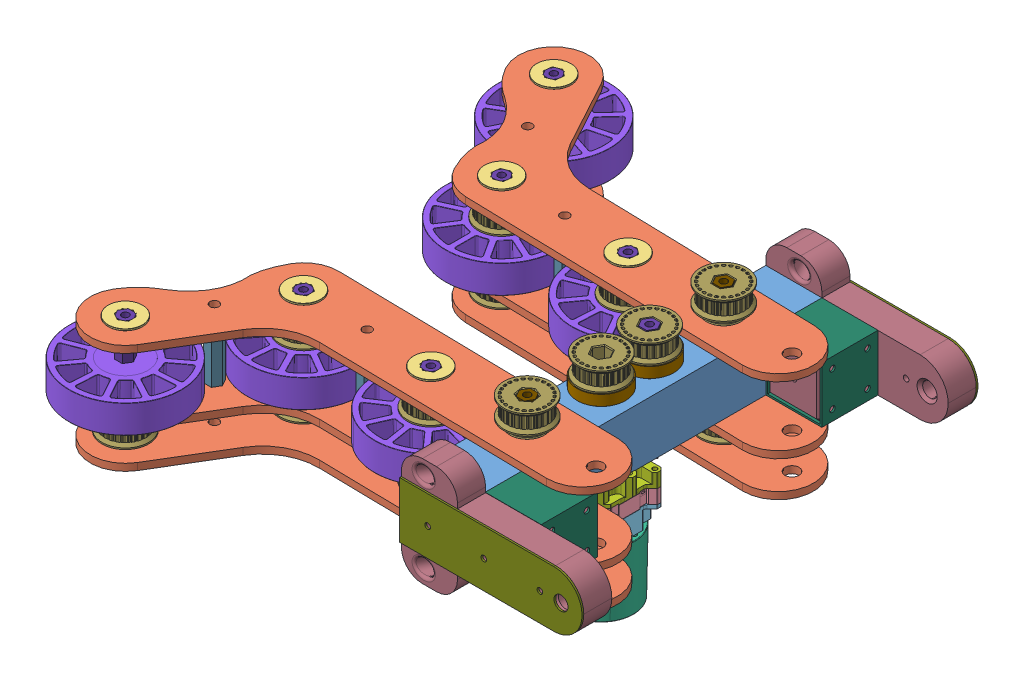
SolidWorks assembly Intake_Claw_1.0, configuration Default. Lengths in mm.
Overall size (476.14 191.6 522.56).
116 component instances, 18 part files, 232 mates.
Components (placement in the parent):
- Claw_Crossbar-1: Claw_Crossbar [Default] at origin size (50.8 50.8 304.8)
- Claw_Intake_Plates-3: Claw_Intake_Plates [Default] at (-63.4848 52.3773 239.6573) x (0.018478 0 -0.999829) z (0.999829 0 0.018478) size (165.24 6.35 379.41)
- am-2986 FR8ZZ Hex Bearing.step-1: am-2986 FR8ZZ Hex Bearing.step [Default] at (25.4 44.3967 241.3) x (-0.023449 0 -0.999725) z (0 1 0) size (31.12 31.12 7.93)
- am-2986 FR8ZZ Hex Bearing.step-3: am-2986 FR8ZZ Hex Bearing.step [Default] at (-241.5471 52.324 338.1202) x (0 0 -1) z (0 1 0) size (31.12 31.12 7.93)
- am-2986 FR8ZZ Hex Bearing.step-5: am-2986 FR8ZZ Hex Bearing.step [Default] at (25.4 52.324 241.3) x (0 0 -1) z (0 1 0) size (31.12 31.12 7.93)
- am-2986 FR8ZZ Hex Bearing.step-11: am-2986 FR8ZZ Hex Bearing.step [Default] at (-63.4848 52.324 239.6573) x (0 0 -1) z (0 1 0) size (31.12 31.12 7.93)
- am-2986 FR8ZZ Hex Bearing.step-12: am-2986 FR8ZZ Hex Bearing.step [Default] at (-180.9398 52.324 237.4866) x (0 0 -1) z (0 1 0) size (31.12 31.12 7.93)
- Intake_Plate_Assembly-1: Intake_Plate_Assembly [Default] at (-25.3851 110.6877 261.8842) x (0.99204 0 0.125922) z (0.125922 0 -0.99204) size (394.05 7.93 202.39)
  - Claw_Intake_Plates-3: Claw_Intake_Plates [Default] at (-63.0534 112.2651 194.2998) x (0.100115 0 -0.994976) z (0.994976 0 0.100115) size (165.24 6.35 379.41)
  - am-2986 FR8ZZ Hex Bearing.step-3: am-2986 FR8ZZ Hex Bearing.step [Default] at (-248.5659 112.2117 277.8835) x (0 0 -1) z (0 1 0) size (31.12 31.12 7.93)
  - am-2986 FR8ZZ Hex Bearing.step-5: am-2986 FR8ZZ Hex Bearing.step [Default] at (25.4 112.2117 203.2) x (0 0 -1) z (0 1 0) size (31.12 31.12 7.93)
  - am-2986 FR8ZZ Hex Bearing.step-11: am-2986 FR8ZZ Hex Bearing.step [Default] at (-63.0534 112.2117 194.2998) x (0 0 -1) z (0 1 0) size (31.12 31.12 7.93)
  - am-2986 FR8ZZ Hex Bearing.step-12: am-2986 FR8ZZ Hex Bearing.step [Default] at (-179.9381 112.2117 182.5388) x (0 0 -1) z (0 1 0) size (31.12 31.12 7.93)
- Intake_Plate_Assembly_2-1: Intake_Plate_Assembly_2 [Default] at (-16.4979 -120.1924 40.8533) x (0.996656 0 -0.081713) z (0.081713 0 0.996656) size (394.05 7.93 202.39)
  - Claw_Intake_Plates-3: Claw_Intake_Plates [Default] at (-63.0746 112.2651 194.2998) x (0.100115 0 -0.994976) z (0.994976 0 0.100115) size (165.24 6.35 379.41)
  - am-2986 FR8ZZ Hex Bearing.step-11: am-2986 FR8ZZ Hex Bearing.step [Default] at (-63.0746 118.6684 194.2998) x (0 0 -1) z (0 -1 0) size (31.12 31.12 7.93)
  - am-2986 FR8ZZ Hex Bearing.step-16: am-2986 FR8ZZ Hex Bearing.step [Default] at (25.3787 118.6684 203.2) x (0 0 -1) z (0 -1 0) size (31.12 31.12 7.93)
  - am-2986 FR8ZZ Hex Bearing.step-17: am-2986 FR8ZZ Hex Bearing.step [Default] at (-179.9594 118.6684 182.5388) x (0 0 -1) z (0 -1 0) size (31.12 31.12 7.93)
  - am-2986 FR8ZZ Hex Bearing.step-18: am-2986 FR8ZZ Hex Bearing.step [Default] at (-248.5872 118.6684 277.8835) x (0 0 -1) z (0 -1 0) size (31.12 31.12 7.93)
- Intake_Plate_Assembly_2-2: Intake_Plate_Assembly_2 [Default] at (-25.364 170.9924 261.8868) x (0.99204 0 0.125922) z (0.125922 0 -0.99204) size (394.05 7.93 202.39)
  - Claw_Intake_Plates-3: Claw_Intake_Plates [Default] at (-63.0746 112.2651 194.2998) x (0.100115 0 -0.994976) z (0.994976 0 0.100115) size (165.24 6.35 379.41)
  - am-2986 FR8ZZ Hex Bearing.step-11: am-2986 FR8ZZ Hex Bearing.step [Default] at (-63.0746 118.6684 194.2998) x (0 0 -1) z (0 -1 0) size (31.12 31.12 7.93)
  - am-2986 FR8ZZ Hex Bearing.step-16: am-2986 FR8ZZ Hex Bearing.step [Default] at (25.3787 118.6684 203.2) x (0 0 -1) z (0 -1 0) size (31.12 31.12 7.93)
  - am-2986 FR8ZZ Hex Bearing.step-17: am-2986 FR8ZZ Hex Bearing.step [Default] at (-179.9594 118.6684 182.5388) x (0 0 -1) z (0 -1 0) size (31.12 31.12 7.93)
  - am-2986 FR8ZZ Hex Bearing.step-18: am-2986 FR8ZZ Hex Bearing.step [Default] at (-248.5872 118.6684 277.8835) x (0 0 -1) z (0 -1 0) size (31.12 31.12 7.93)
- REV-21-2103.step-1: REV-21-2103.step [Default] at (25.4 -25.0519 174.244) x (1 0 0) z (0 1 0) size (61.91 50.8 16.85)
- REV-21-2106.step-1: REV-21-2106.step [Default] at (25.4 -40.9269 174.244) x (1 0 0) z (0 1 0) size (61.91 50.8 19.05)
- REV-21-1650-V1.1.step-1: REV-21-1650-V1.1.step [Default] at (25.4 -50.4519 174.244) x (0.832107 0 0.554615) z (0 1 0) size (68.13 68.01 93.35)
- REV-21-2104.step-1: REV-21-2104.step [Default] at (25.4 -9.1769 174.244) x (0 1 0) z (-1 0 0) size (23.2 50.8 61.92)
- am-3480 4IN 500Hex Bore Compliant Wheel REV2.STEP-1: am-3480 4IN 500Hex Bore Compliant Wheel REV2.STEP [Default] at (-229.2406 20.303 326.8494) x (0.873407 0 -0.486991) z (0 -1 0) size (101.6 101.6 25.4)
- am-3480 4IN 500Hex Bore Compliant Wheel REV2.STEP-2: am-3480 4IN 500Hex Bore Compliant Wheel REV2.STEP [Default] at (-176.0869 20.303 221.52) x (0.503742 0 -0.863854) z (0 -1 0) size (101.6 101.6 25.4)
- am-3480 4IN 500Hex Bore Compliant Wheel REV2.STEP-3: am-3480 4IN 500Hex Bore Compliant Wheel REV2.STEP [Default] at (-68.7896 20.303 255.4796) x (-0.528092 0 0.849187) z (0 -1 0) size (101.6 101.6 25.4)
- am-3480 4IN 500Hex Bore Compliant Wheel REV2.STEP-4: am-3480 4IN 500Hex Bore Compliant Wheel REV2.STEP [Default] at (-47.0349 20.303 58.2982) x (0.998282 0 0.058584) z (0 -1 0) size (101.6 101.6 25.4)
- am-3480 4IN 500Hex Bore Compliant Wheel REV2.STEP-5: am-3480 4IN 500Hex Bore Compliant Wheel REV2.STEP [Default] at (-164.668 20.303 54.2894) x (1 0 0) z (0 -1 0) size (101.6 101.6 25.4)
- am-3480 4IN 500Hex Bore Compliant Wheel REV2.STEP-6: am-3480 4IN 500Hex Bore Compliant Wheel REV2.STEP [Default] at (-244.8133 20.303 -59.8228) x (-0.252916 0 -0.967488) z (0 -1 0) size (101.6 101.6 25.4)
- am-2986 FR8ZZ Hex Bearing.step-13: am-2986 FR8ZZ Hex Bearing.step [Default] at (25.4 6.4033 130.556) x (-0.368447 0 0.929649) z (0 -1 0) size (31.12 31.12 7.93)
- am-2986 FR8ZZ Hex Bearing.step-14: am-2986 FR8ZZ Hex Bearing.step [Default] at (25.4 44.3967 130.556) x (-0.368447 0 0.929649) z (0 1 0) size (31.12 31.12 7.93)
- am-2986 FR8ZZ Hex Bearing.step-15: am-2986 FR8ZZ Hex Bearing.step [Default] at (25.4 44.3967 174.244) x (-0.368447 0 0.929649) z (0 1 0) size (31.12 31.12 7.93)
- Claw_Drive_Gear-1: Claw_Drive_Gear [Default] at (25.4 55.499 130.556) x (0.998817 0 0.048625) z (-0.048625 0 0.998817) size (43.69 9.45 43.69)
- Claw_Drive_Gear-2: Claw_Drive_Gear [Default] at (25.4 55.499 174.244) x (0.998302 0 -0.058242) z (0.058242 0 0.998302) size (43.69 9.45 43.69)
- half_inch_hex_spacer_0.125inch-1: half_inch_hex_spacer_0.125inch [Default] at (25.4 52.324 130.556) x (0.999916 0 -0.012929) z (0.012929 0 0.999916) size (20.32 3.17 20.32)
- half_inch_hex_spacer_0.125inch-2: half_inch_hex_spacer_0.125inch [Default] at (25.4 52.324 174.244) x (0.999469 0 0.032576) z (-0.032576 0 0.999469) size (20.32 3.17 20.32)
- am-2986 FR8ZZ Hex Bearing.step-16: am-2986 FR8ZZ Hex Bearing.step [Default] at (25.4 44.3967 63.5) x (-0.023449 0 -0.999725) z (0 1 0) size (31.12 31.12 7.93)
- am-2986 FR8ZZ Hex Bearing.step-18: am-2986 FR8ZZ Hex Bearing.step [Default] at (25.4 6.4033 63.5) x (-0.368447 0 0.929649) z (0 -1 0) size (31.12 31.12 7.93)
- am-2986 FR8ZZ Hex Bearing.step-19: am-2986 FR8ZZ Hex Bearing.step [Default] at (25.4 6.4033 241.3) x (-0.368447 0 0.929649) z (0 -1 0) size (31.12 31.12 7.93)
- half_inch_hex_spacer_0.1875inch-1: half_inch_hex_spacer_0.1875inch [Default] at (25.4 60.2513 63.5) size (20.32 4.76 20.32)
- half_inch_hex_spacer_0.1875inch-2: half_inch_hex_spacer_0.1875inch [Default] at (25.4 60.2513 241.3) size (20.32 4.76 20.32)
- 24_tooth_5mmHTD_timing_belt_pulley_9mm-3: 24_tooth_5mmHTD_timing_belt_pulley_9mm [Default] at (-180.9398 30.861 237.4866) x (0.987086 0 0.160191) z (0 -1 0) size (42.16 42.16 17.78)
- 24_tooth_5mmHTD_timing_belt_pulley_9mm-7: 24_tooth_5mmHTD_timing_belt_pulley_9mm [Default] at (25.4 68.8238 241.3) x (0.782455 0 -0.622708) z (0 -1 0) size (42.16 42.16 17.78)
- 24_tooth_5mmHTD_timing_belt_pulley_9mm-8: 24_tooth_5mmHTD_timing_belt_pulley_9mm [Default] at (25.4 68.7578 174.244) x (1 0 0) z (0 -1 0) size (42.16 42.16 17.78)
- 24_tooth_5mmHTD_timing_belt_pulley_9mm-9: 24_tooth_5mmHTD_timing_belt_pulley_9mm [Default] at (25.4 68.7578 130.556) x (1 0 0) z (0 -1 0) size (42.16 42.16 17.78)
- 24_tooth_5mmHTD_timing_belt_pulley_9mm-10: 24_tooth_5mmHTD_timing_belt_pulley_9mm [Default] at (25.4 68.8238 63.5) x (1 0 0) z (0 -1 0) size (42.16 42.16 17.78)
- 24_tooth_5mmHTD_timing_belt_pulley_9mm-13: 24_tooth_5mmHTD_timing_belt_pulley_9mm [Default] at (-180.9054 30.861 58.1403) x (0.911482 0 -0.411341) z (0 -1 0) size (42.16 42.16 17.78)
- 24_tooth_5mmHTD_timing_belt_pulley_9mm-15: 24_tooth_5mmHTD_timing_belt_pulley_9mm [Default] at (-63.4848 30.861 239.6573) x (0.911482 0 -0.411341) z (0 -1 0) size (42.16 42.16 17.78)
- 24_tooth_5mmHTD_timing_belt_pulley_9mm-16: 24_tooth_5mmHTD_timing_belt_pulley_9mm [Default] at (-63.47 30.861 61.1912) x (0.84545 0 -0.534054) z (0 -1 0) size (42.16 42.16 17.78)
- half_inch_hex_spacer_0.125inch-13: half_inch_hex_spacer_0.125inch [Default] at (-63.47 -1.524 61.1912) size (20.32 3.17 20.32)
- half_inch_hex_spacer_0.125inch-14: half_inch_hex_spacer_0.125inch [Default] at (-180.9054 -1.524 58.1403) size (20.32 3.17 20.32)
- half_inch_hex_spacer_0.125inch-15: half_inch_hex_spacer_0.125inch [Default] at (-236.9809 -1.524 -45.0872) size (20.32 3.17 20.32)
- half_inch_hex_spacer_0.125inch-16: half_inch_hex_spacer_0.125inch [Default] at (-63.4848 -1.524 239.6573) size (20.32 3.17 20.32)
- half_inch_hex_spacer_0.125inch-17: half_inch_hex_spacer_0.125inch [Default] at (-180.9398 -1.524 237.4866) size (20.32 3.17 20.32)
- half_inch_hex_spacer_0.125inch-18: half_inch_hex_spacer_0.125inch [Default] at (-241.5471 -1.524 338.1202) size (20.32 3.17 20.32)
- Grabber_Spring_Mount-1: Grabber_Spring_Mount [Default] at (49.2125 48.8315 254) x (-1 0 0) z (0 0 1) size (165.1 98.04 76.2)
- Grabber_Spring_Mount-2: Grabber_Spring_Mount [Default] at (48.8315 1.5875 50.8) x (-1 0 0) z (0 0 -1) size (165.1 98.04 76.2)
- 24_tooth_5mmHTD_timing_belt_pulley_9mm-17: 24_tooth_5mmHTD_timing_belt_pulley_9mm [Default] at (25.4 -26.5963 241.3) x (0.782455 0 -0.622708) z (0 -1 0) size (42.16 42.16 17.78)
- 24_tooth_5mmHTD_timing_belt_pulley_9mm-18: 24_tooth_5mmHTD_timing_belt_pulley_9mm [Default] at (25.4 -26.5963 63.5) x (0.782455 0 -0.622708) z (0 -1 0) size (42.16 42.16 17.78)
- half_inch_hex_spacer_0.125inch-19: half_inch_hex_spacer_0.125inch [Default] at (25.4 -12.6263 63.5) size (20.32 3.17 20.32)
- half_inch_hex_spacer_0.125inch-20: half_inch_hex_spacer_0.125inch [Default] at (25.4 -12.6263 241.3) size (20.32 3.17 20.32)
- half_inch_hex_spacer_0.125inch-21: half_inch_hex_spacer_0.125inch [Default] at (-63.47 -12.6263 61.1912) size (20.32 3.17 20.32)
- half_inch_hex_spacer_0.125inch-22: half_inch_hex_spacer_0.125inch [Default] at (-180.9054 -12.6263 58.1403) size (20.32 3.17 20.32)
- half_inch_hex_spacer_0.125inch-23: half_inch_hex_spacer_0.125inch [Default] at (-236.9809 -12.6263 -45.0872) size (20.32 3.17 20.32)
- half_inch_hex_spacer_0.125inch-24: half_inch_hex_spacer_0.125inch [Default] at (-241.5471 -12.6263 338.1202) size (20.32 3.17 20.32)
- half_inch_hex_spacer_0.125inch-25: half_inch_hex_spacer_0.125inch [Default] at (-180.9398 -12.6263 237.4866) size (20.32 3.17 20.32)
- half_inch_hex_spacer_0.125inch-26: half_inch_hex_spacer_0.125inch [Default] at (-63.4848 -12.6263 239.6573) size (20.32 3.17 20.32)
- half_inch_hex_spacer_0.125inch-27: half_inch_hex_spacer_0.125inch [Default] at (-63.4848 -33.5813 239.6573) size (20.32 3.17 20.32)
- half_inch_hex_spacer_0.125inch-28: half_inch_hex_spacer_0.125inch [Default] at (-180.9398 -33.5813 237.4866) size (20.32 3.17 20.32)
- half_inch_hex_spacer_0.125inch-29: half_inch_hex_spacer_0.125inch [Default] at (-241.5471 -33.5813 338.1202) size (20.32 3.17 20.32)
- half_inch_hex_spacer_0.125inch-30: half_inch_hex_spacer_0.125inch [Default] at (-63.47 -33.5813 61.1912) size (20.32 3.17 20.32)
- half_inch_hex_spacer_0.125inch-31: half_inch_hex_spacer_0.125inch [Default] at (-180.9054 -33.5813 58.1403) size (20.32 3.17 20.32)
- half_inch_hex_spacer_0.125inch-32: half_inch_hex_spacer_0.125inch [Default] at (-236.9809 -33.5813 -45.0872) size (20.32 3.17 20.32)
- 24_tooth_5mmHTD_timing_belt_pulley_9mm-19: 24_tooth_5mmHTD_timing_belt_pulley_9mm [Default] at (-63.47 -26.5963 61.1912) x (1 0 0) z (0 -1 0) size (42.16 42.16 17.78)
- 24_tooth_5mmHTD_timing_belt_pulley_9mm-20: 24_tooth_5mmHTD_timing_belt_pulley_9mm [Default] at (-180.9054 -26.5963 58.1403) x (1 0 0) z (0 -1 0) size (42.16 42.16 17.78)
- 24_tooth_5mmHTD_timing_belt_pulley_9mm-21: 24_tooth_5mmHTD_timing_belt_pulley_9mm [Default] at (-236.9809 -26.5963 -45.0872) x (1 0 0) z (0 -1 0) size (42.16 42.16 17.78)
- 24_tooth_5mmHTD_timing_belt_pulley_9mm-22: 24_tooth_5mmHTD_timing_belt_pulley_9mm [Default] at (-241.5471 -26.5963 338.1202) x (1 0 0) z (0 -1 0) size (42.16 42.16 17.78)
- 24_tooth_5mmHTD_timing_belt_pulley_9mm-23: 24_tooth_5mmHTD_timing_belt_pulley_9mm [Default] at (-180.9398 -26.5963 237.4866) x (1 0 0) z (0 -1 0) size (42.16 42.16 17.78)
- 24_tooth_5mmHTD_timing_belt_pulley_9mm-24: 24_tooth_5mmHTD_timing_belt_pulley_9mm [Default] at (-63.4848 -26.5963 239.6573) x (1 0 0) z (0 -1 0) size (42.16 42.16 17.78)
- half_inch_hex_spacer_0.125inch-33: half_inch_hex_spacer_0.125inch [Default] at (25.4 -33.5813 63.5) size (20.32 3.17 20.32)
- half_inch_hex_spacer_0.125inch-34: half_inch_hex_spacer_0.125inch [Default] at (25.4 -33.5813 241.3) size (20.32 3.17 20.32)
- Intake_Plate_Assembly-3: Intake_Plate_Assembly [Default] at (-25.3851 78.6304 261.8842) x (0.99204 0 0.125922) z (0.125922 0 -0.99204) size (394.05 7.93 202.39)
  - Claw_Intake_Plates-3: Claw_Intake_Plates [Default] at (-63.0534 112.2651 194.2998) x (0.100115 0 -0.994976) z (0.994976 0 0.100115) size (165.24 6.35 379.41)
  - am-2986 FR8ZZ Hex Bearing.step-3: am-2986 FR8ZZ Hex Bearing.step [Default] at (-248.5659 112.2117 277.8835) x (0 0 -1) z (0 1 0) size (31.12 31.12 7.93)
  - am-2986 FR8ZZ Hex Bearing.step-5: am-2986 FR8ZZ Hex Bearing.step [Default] at (25.4 112.2117 203.2) x (0 0 -1) z (0 1 0) size (31.12 31.12 7.93)
  - am-2986 FR8ZZ Hex Bearing.step-11: am-2986 FR8ZZ Hex Bearing.step [Default] at (-63.0534 112.2117 194.2998) x (0 0 -1) z (0 1 0) size (31.12 31.12 7.93)
  - am-2986 FR8ZZ Hex Bearing.step-12: am-2986 FR8ZZ Hex Bearing.step [Default] at (-179.9381 112.2117 182.5388) x (0 0 -1) z (0 1 0) size (31.12 31.12 7.93)
- Intake_Plate_Assembly_2-4: Intake_Plate_Assembly_2 [Default] at (-16.4979 -152.2498 40.8533) x (0.996656 0 -0.081713) z (0.081713 0 0.996656) size (394.05 7.93 202.39)
  - Claw_Intake_Plates-3: Claw_Intake_Plates [Default] at (-63.0746 112.2651 194.2998) x (0.100115 0 -0.994976) z (0.994976 0 0.100115) size (165.24 6.35 379.41)
  - am-2986 FR8ZZ Hex Bearing.step-11: am-2986 FR8ZZ Hex Bearing.step [Default] at (-63.0746 118.6684 194.2998) x (0 0 -1) z (0 -1 0) size (31.12 31.12 7.93)
  - am-2986 FR8ZZ Hex Bearing.step-16: am-2986 FR8ZZ Hex Bearing.step [Default] at (25.3787 118.6684 203.2) x (0 0 -1) z (0 -1 0) size (31.12 31.12 7.93)
  - am-2986 FR8ZZ Hex Bearing.step-17: am-2986 FR8ZZ Hex Bearing.step [Default] at (-179.9594 118.6684 182.5388) x (0 0 -1) z (0 -1 0) size (31.12 31.12 7.93)
  - am-2986 FR8ZZ Hex Bearing.step-18: am-2986 FR8ZZ Hex Bearing.step [Default] at (-248.5872 118.6684 277.8835) x (0 0 -1) z (0 -1 0) size (31.12 31.12 7.93)
- grabber_stand_off-1: grabber_stand_off [Default] at (-122.2123 52.3977 238.572) x (1 0 0) z (0 -1 0) size (14.66 12.7 53.98)
- grabber_stand_off-3: grabber_stand_off [Default] at (-211.2434 52.3773 287.8034) x (1 0 0) z (0 -1 0) size (14.66 12.7 53.98)
- grabber_stand_off-4: grabber_stand_off [Default] at (-208.9431 52.3773 6.5265) x (-0.606361 0 0.795189) z (0 -1 0) size (14.66 12.7 53.98)
- grabber_stand_off-5: grabber_stand_off [Default] at (-122.1877 52.3773 59.6657) x (1 0 0) z (0 -1 0) size (14.66 12.7 53.98)
- Crossbar_Bracket-1: Crossbar_Bracket [Default] at (101.6 0 0) x (0 1 0) z (0 0 1) size (50.8 50.8 50.8)
- Crossbar_Bracket-2: Crossbar_Bracket [Default] at (101.6 0 254) x (0 1 0) z (0 0 1) size (50.8 50.8 50.8)
- Claw_Pivot_Plate-1: Claw_Pivot_Plate [Default] at (0.381 -0.1905 330.2) size (165.1 50.8 1.59)
- Claw_Pivot_Plate-2: Claw_Pivot_Plate [Default] at (0 -0.1905 -26.9875) size (165.1 50.8 1.59)
- grabber_wheel_axle-1: grabber_wheel_axle [Default] at (-236.9809 60.2513 -45.0872) x (1 0 0) z (0 -1 0) size (14.66 12.7 101.6)
- grabber_wheel_axle-2: grabber_wheel_axle [Default] at (-180.9054 60.2513 58.1403) x (1 0 0) z (0 -1 0) size (14.66 12.7 101.6)
- grabber_wheel_axle-3: grabber_wheel_axle [Default] at (-63.47 60.2513 61.1912) x (1 0 0) z (0 -1 0) size (14.66 12.7 101.6)
- grabber_wheel_axle-4: grabber_wheel_axle [Default] at (25.4 82.7278 130.556) x (1 0 0) z (0 -1 0) size (14.66 12.7 101.6)
- grabber_wheel_axle-5: grabber_wheel_axle [Default] at (-241.5471 60.2513 338.1202) x (1 0 0) z (0 -1 0) size (14.66 12.7 101.6)
- grabber_wheel_axle-6: grabber_wheel_axle [Default] at (-180.9398 60.2513 237.4866) x (1 0 0) z (0 -1 0) size (14.66 12.7 101.6)
- grabber_wheel_axle-7: grabber_wheel_axle [Default] at (-63.4848 60.2513 239.6573) x (1 0 0) z (0 -1 0) size (14.66 12.7 101.6)
- grabber_pivot_axle-1: grabber_pivot_axle [Default] at (25.4 82.7938 63.5) x (1 0 0) z (0 -1 0) size (14.66 12.7 126.33)
- grabber_pivot_axle-2: grabber_pivot_axle [Default] at (25.4 82.7938 241.3) x (1 0 0) z (0 -1 0) size (14.66 12.7 126.33)
Mates (geometry in assembly coordinates):
- Concentric2: concentric aligned: circle of Claw_Crossbar-1; circle of Claw_Intake_Plates-3
- Concentric5: concentric aligned: circle of Claw_Crossbar-1; circle of am-2986 FR8ZZ Hex Bearing.step-1
- Coincident11: coincident anti-aligned: plane of Claw_Crossbar-1 through (0 50.8 304.8) normal (0 1 0); plane of am-2986 FR8ZZ Hex Bearing.step-1 through (25.0724 50.8 227.3338) normal (0 -1 0)
- Concentric6: concentric anti-aligned: cylinder of Claw_Intake_Plates-3; cylinder of am-2986 FR8ZZ Hex Bearing.step-5 through (25.4 60.2513 241.3) axis (0 -1 0) radius 15.5575
- Coincident12: coincident anti-aligned: plane of Claw_Intake_Plates-3 through (-241.5471 58.7273 338.1202) normal (0 1 0); plane of am-2986 FR8ZZ Hex Bearing.step-5 through (25.4 58.7273 227.33) normal (0 -1 0)
- Concentric7: concentric aligned: circle of Claw_Intake_Plates-3; circle of am-2986 FR8ZZ Hex Bearing.step-11
- Coincident13: coincident anti-aligned: plane of Claw_Intake_Plates-3 through (-241.5471 58.7273 338.1202) normal (0 1 0); plane of am-2986 FR8ZZ Hex Bearing.step-11 through (-63.4848 58.7273 225.6873) normal (0 -1 0)
- Concentric8: concentric aligned: circle of Claw_Intake_Plates-3; circle of am-2986 FR8ZZ Hex Bearing.step-12
- Coincident14: coincident anti-aligned: plane of Claw_Intake_Plates-3 through (-241.5471 58.7273 338.1202) normal (0 1 0); plane of am-2986 FR8ZZ Hex Bearing.step-12 through (-180.9398 58.7273 223.5166) normal (0 -1 0)
- Concentric9: concentric aligned: circle of Claw_Intake_Plates-3; circle of am-2986 FR8ZZ Hex Bearing.step-3
- Coincident15: coincident anti-aligned: plane of Claw_Intake_Plates-3 through (-241.5471 58.7273 338.1202) normal (0 1 0); plane of am-2986 FR8ZZ Hex Bearing.step-3 through (-241.5471 58.7273 324.1502) normal (0 -1 0)
- Concentric10: concentric anti-aligned: circle of Claw_Crossbar-1; circle of Intake_Plate_Assembly-1/am-2986 FR8ZZ Hex Bearing.step-5
- Concentric11: concentric aligned: circle of Claw_Crossbar-1; circle of Intake_Plate_Assembly_2-1/Claw_Intake_Plates-3
- Concentric12: concentric anti-aligned: circle of Claw_Crossbar-1; circle of Intake_Plate_Assembly_2-2/Claw_Intake_Plates-3
- Parallel3: parallel aligned: plane of Intake_Plate_Assembly-1/Claw_Intake_Plates-3 through (77.0074 -7.9273 33.08) normal (0.025971 0 -0.999663); plane of Intake_Plate_Assembly_2-2/Claw_Intake_Plates-3 through (77.0074 52.3773 33.08) normal (0.025971 0 -0.999663)
- Parallel4: parallel aligned: plane of Claw_Intake_Plates-3 through (75.6047 58.7273 273.9833) normal (-0.018478 0 0.999829); plane of Intake_Plate_Assembly_2-1/Claw_Intake_Plates-3 through (75.6047 -1.5773 273.9833) normal (-0.018478 0 0.999829)
- Concentric13: concentric anti-aligned: circle of REV-21-2106.step-1; circle of REV-21-1650-V1.1.step-1
- Coincident16: coincident anti-aligned: plane of REV-21-2106.step-1 through (25.4 -50.4519 174.244) normal (0 -1 0); plane of REV-21-1650-V1.1.step-1 through (25.4 -50.4519 174.244) normal (0 1 0)
- Concentric14: concentric aligned: circle of REV-21-2103.step-1; circle of REV-21-2106.step-1
- Coincident17: coincident anti-aligned: plane of REV-21-2103.step-1 through (25.4 -31.4019 174.244) normal (0 -1 0); plane of REV-21-2106.step-1 through (25.4 -31.4019 174.244) normal (0 1 0)
- Concentric15: concentric anti-aligned: circle of REV-21-1650-V1.1.step-1; circle of REV-21-2104.step-1
- Coincident18: coincident anti-aligned: plane of REV-21-2103.step-1 through (25.4 -18.7019 174.244) normal (0 1 0); plane of REV-21-2104.step-1 through (25.4 -18.7019 174.244) normal (0 -1 0)
- Coincident19: coincident aligned: plane of REV-21-2103.step-1 through (50.8 -18.7019 148.844) normal (0 0 -1); plane of REV-21-2104.step-1 through (50.8 -18.7019 148.844) normal (0 0 -1)
- Coincident20: coincident aligned: plane of REV-21-2103.step-1 through (50.8 -18.7019 148.844) normal (0 0 -1); plane of REV-21-2106.step-1 through (25.4 -31.4019 148.844) normal (0 0 -1)
- Concentric16: concentric anti-aligned: circle of REV-21-2106.step-1; circle of REV-21-1650-V1.1.step-1
- Concentric17: concentric anti-aligned: circle of Intake_Plate_Assembly_2-1/am-2986 FR8ZZ Hex Bearing.step-18; circle of am-3480 4IN 500Hex Bore Compliant Wheel REV2.STEP-1
- Concentric18: concentric anti-aligned: circle of Intake_Plate_Assembly_2-1/am-2986 FR8ZZ Hex Bearing.step-17; circle of am-3480 4IN 500Hex Bore Compliant Wheel REV2.STEP-2
- Concentric20: concentric anti-aligned: circle of Intake_Plate_Assembly-1/am-2986 FR8ZZ Hex Bearing.step-12; circle of am-3480 4IN 500Hex Bore Compliant Wheel REV2.STEP-5
- Concentric21: concentric aligned: circle of Intake_Plate_Assembly-1/am-2986 FR8ZZ Hex Bearing.step-11; circle of am-3480 4IN 500Hex Bore Compliant Wheel REV2.STEP-4
- Concentric22: concentric anti-aligned: circle of Intake_Plate_Assembly-1/am-2986 FR8ZZ Hex Bearing.step-3; circle of am-3480 4IN 500Hex Bore Compliant Wheel REV2.STEP-6
- Coincident21: coincident aligned: plane of am-3480 4IN 500Hex Bore Compliant Wheel REV2.STEP-5 through (-180.9054 1.651 78.6518) normal (0 -1 0); plane of am-3480 4IN 500Hex Bore Compliant Wheel REV2.STEP-6 through (-217.1363 1.651 -50.2749) normal (0 -1 0)
- Coincident22: coincident aligned: plane of am-3480 4IN 500Hex Bore Compliant Wheel REV2.STEP-4 through (-64.6717 1.651 81.6675) normal (0 -1 0); plane of am-3480 4IN 500Hex Bore Compliant Wheel REV2.STEP-5 through (-180.9054 1.651 78.6518) normal (0 -1 0)
- Coincident23: coincident aligned: plane of am-3480 4IN 500Hex Bore Compliant Wheel REV2.STEP-2 through (-163.2208 1.651 247.8191) normal (0 -1 0); plane of am-3480 4IN 500Hex Bore Compliant Wheel REV2.STEP-4 through (-64.6717 1.651 81.6675) normal (0 -1 0)
- Coincident24: coincident aligned: plane of am-3480 4IN 500Hex Bore Compliant Wheel REV2.STEP-1 through (-231.5582 1.651 356.0351) normal (0 -1 0); plane of am-3480 4IN 500Hex Bore Compliant Wheel REV2.STEP-2 through (-163.2208 1.651 247.8191) normal (0 -1 0)
- Coincident25: coincident aligned: plane of am-3480 4IN 500Hex Bore Compliant Wheel REV2.STEP-1 through (-231.5582 1.651 356.0351) normal (0 -1 0); plane of am-3480 4IN 500Hex Bore Compliant Wheel REV2.STEP-3 through (-80.9029 1.651 228.8254) normal (0 -1 0)
- Concentric23: concentric anti-aligned: circle of Intake_Plate_Assembly_2-1/am-2986 FR8ZZ Hex Bearing.step-11; circle of am-3480 4IN 500Hex Bore Compliant Wheel REV2.STEP-3
- Coincident26: coincident aligned: plane of Intake_Plate_Assembly-1/Claw_Intake_Plates-3 through (-236.9809 -7.9273 -45.0872) normal (0 -1 0); plane of Intake_Plate_Assembly_2-1/Claw_Intake_Plates-3 through (-241.5471 -7.9273 338.1202) normal (0 -1 0)
- Coincident27: coincident aligned: plane of Claw_Intake_Plates-3 through (-241.5471 52.3773 338.1202) normal (0 -1 0); plane of Intake_Plate_Assembly_2-2/Claw_Intake_Plates-3 through (-236.9809 52.3773 -45.0872) normal (0 -1 0)
- Parallel6: parallel aligned: plane of Claw_Crossbar-1 through (50.8 0 304.8) normal (1 0 0); plane of REV-21-2103.step-1 through (50.8 -18.7019 199.644) normal (1 0 0)
- Concentric25: concentric anti-aligned: circle of Claw_Crossbar-1; circle of REV-21-2104.step-1
- Concentric26: concentric anti-aligned: circle of Claw_Crossbar-1; circle of am-2986 FR8ZZ Hex Bearing.step-13
- Coincident30: coincident anti-aligned: plane of Claw_Crossbar-1 through (0 0 304.8) normal (0 -1 0); plane of am-2986 FR8ZZ Hex Bearing.step-13 through (20.2528 0 143.5432) normal (0 1 0)
- Concentric27: concentric anti-aligned: circle of Claw_Crossbar-1; circle of am-2986 FR8ZZ Hex Bearing.step-14
- Concentric28: concentric anti-aligned: circle of Claw_Crossbar-1; circle of am-2986 FR8ZZ Hex Bearing.step-15
- Coincident31: coincident anti-aligned: plane of Claw_Crossbar-1 through (0 50.8 304.8) normal (0 1 0); plane of am-2986 FR8ZZ Hex Bearing.step-15 through (20.2528 50.8 187.2312) normal (0 -1 0)
- Coincident32: coincident anti-aligned: plane of Claw_Crossbar-1 through (0 50.8 304.8) normal (0 1 0); plane of am-2986 FR8ZZ Hex Bearing.step-14 through (20.2528 50.8 143.5432) normal (0 -1 0)
- Concentric29: concentric aligned: circle of am-2986 FR8ZZ Hex Bearing.step-14; circle of Claw_Drive_Gear-1
- Concentric30: concentric anti-aligned: circle of am-2986 FR8ZZ Hex Bearing.step-15; circle of Claw_Drive_Gear-2
- Concentric31: concentric anti-aligned: circle of am-2986 FR8ZZ Hex Bearing.step-14; circle of half_inch_hex_spacer_0.125inch-1
- Concentric32: concentric anti-aligned: circle of am-2986 FR8ZZ Hex Bearing.step-15; circle of half_inch_hex_spacer_0.125inch-2
- Coincident33: coincident anti-aligned: plane of am-2986 FR8ZZ Hex Bearing.step-14 through (19.6679 52.324 145.019) normal (0 1 0); plane of half_inch_hex_spacer_0.125inch-1 through (25.4 52.324 130.556) normal (0 -1 0)
- Coincident34: coincident anti-aligned: plane of am-2986 FR8ZZ Hex Bearing.step-15 through (19.6679 52.324 188.707) normal (0 1 0); plane of half_inch_hex_spacer_0.125inch-2 through (25.4 52.324 174.244) normal (0 -1 0)
- Coincident35: coincident anti-aligned: plane of Claw_Drive_Gear-1 through (25.4 55.499 130.556) normal (0 -1 0); plane of half_inch_hex_spacer_0.125inch-1 through (25.4 55.499 130.556) normal (0 1 0)
- Coincident36: coincident anti-aligned: plane of Claw_Drive_Gear-2 through (25.4 55.499 174.244) normal (0 -1 0); plane of half_inch_hex_spacer_0.125inch-2 through (25.4 55.499 174.244) normal (0 1 0)
- Coincident37: coincident anti-aligned: plane of Claw_Drive_Gear-1 through (25.4 64.9478 130.556) normal (0 1 0); plane of half_inch_hex_spacer_0.125inch-3 through (25.4 64.9478 130.556) normal (0 -1 0)
- Concentric33: concentric aligned: circle of Claw_Drive_Gear-1; circle of half_inch_hex_spacer_0.125inch-3
- Coincident38: coincident anti-aligned: plane of Claw_Drive_Gear-2 through (25.4 64.9478 174.244) normal (0 1 0); plane of half_inch_hex_spacer_0.125inch-4 through (25.4 64.9478 174.244) normal (0 -1 0)
- Concentric34: concentric aligned: circle of Claw_Drive_Gear-2; circle of half_inch_hex_spacer_0.125inch-4
- Coincident39: coincident anti-aligned: plane of Claw_Crossbar-1 through (0 50.8 304.8) normal (0 1 0); plane of am-2986 FR8ZZ Hex Bearing.step-16 through (25.0724 50.8 49.5338) normal (0 -1 0)
- Concentric35: concentric anti-aligned: circle of Claw_Crossbar-1; circle of am-2986 FR8ZZ Hex Bearing.step-16
- Coincident40: coincident anti-aligned: plane of Claw_Crossbar-1 through (0 0 304.8) normal (0 -1 0); plane of am-2986 FR8ZZ Hex Bearing.step-18 through (20.2528 0 76.4872) normal (0 1 0)
- Coincident41: coincident anti-aligned: plane of Claw_Crossbar-1 through (0 0 304.8) normal (0 -1 0); plane of am-2986 FR8ZZ Hex Bearing.step-19 through (20.2528 0 254.2872) normal (0 1 0)
- Concentric36: concentric anti-aligned: circle of Claw_Crossbar-1; circle of am-2986 FR8ZZ Hex Bearing.step-19
- Concentric37: concentric anti-aligned: circle of Claw_Crossbar-1; circle of am-2986 FR8ZZ Hex Bearing.step-18
- Coincident42: coincident anti-aligned: plane of Intake_Plate_Assembly_2-1/am-2986 FR8ZZ Hex Bearing.step-16 through (25.4 -1.524 241.3) normal (0 1 0); plane of am-2986 FR8ZZ Hex Bearing.step-19 through (19.6679 -1.524 255.763) normal (0 -1 0)
- Coincident43: coincident anti-aligned: plane of am-2986 FR8ZZ Hex Bearing.step-1 through (25.0352 52.324 225.7468) normal (0 1 0); plane of am-2986 FR8ZZ Hex Bearing.step-5 through (25.4 52.324 241.3) normal (0 -1 0)
- Coincident45: coincident anti-aligned: plane of Claw_Drive_Gear-1 through (25.4 64.9478 130.556) normal (0 1 0); plane of 18_tooth_5mmHTD_timing_belt_pulley_9mm-1 through (25.4 64.9478 130.556) normal (0 -1 0)
- Concentric39: concentric aligned: circle of Claw_Drive_Gear-1; circle of 18_tooth_5mmHTD_timing_belt_pulley_9mm-1
- Parallel7: parallel anti-aligned: plane of Claw_Drive_Gear-2 through (25.4 55.499 174.244) normal (0 -1 0); plane of half_inch_hex_spacer_0.125inch-4 through (25.4 68.1228 174.244) normal (0 1 0)
